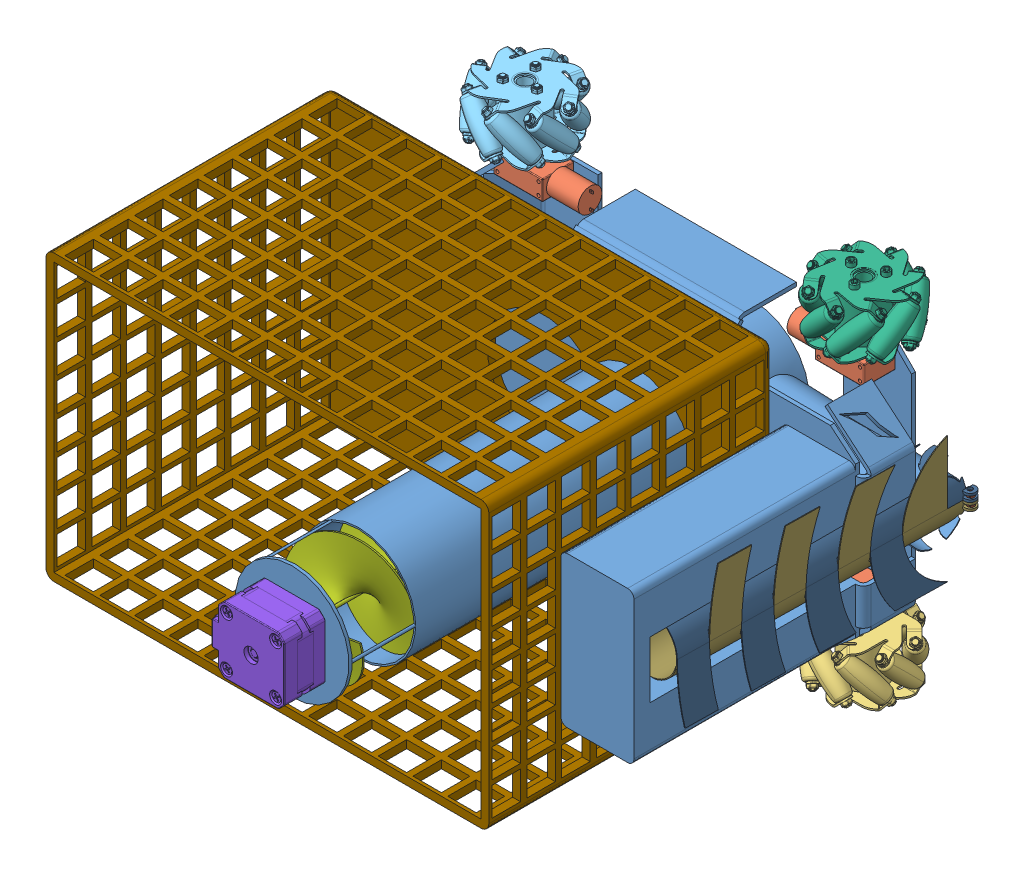
SolidWorks assembly tennis_car2, configuration 默认. Lengths in mm.
Overall size (342.44 226.19 334.2).
20 component instances, 12 part files, 28 mates.
Components (placement in the parent):
- car_main_body-1: car_main_body [默认] at (-145.051 -370.0736 71.4729) x (0 1 0) z (0 0 1) size (155.3 280.48 291.54)
- RF-1: RF [默认] at (73.9859 -396.0617 -100.86) size (72.83 55.75 59.47)
  - DC-1: DC [默认] at (11.5455 -40.5143 8.3808) x (-1 0 0) z (0 -1 0) size (53.09 20 29.75)
  - Mecanum_wheel_RF-1: Mecanum_wheel_RF [默认] at (50.073 -104.5143 -58.7387) x (0 1 0) z (0 0 1) size (37 59.47 59.47)
- RB-1: RB [默认] at (-99.6113 -409.5895 -127.3135) size (85.22 55.84 84.26)
  - DC-1: DC [默认] at (0.8482 -26.9825 34.8343) x (1 0 0) z (0 -1 0) size (53.09 20 29.75)
  - Mecanum_wheel_RB2-1: Mecanum_wheel_RB2 [默认] at (-29.583 -87.0073 9.2199) x (0 -1 0) z (0.536613 0 0.843828) size (37 61.04 61.04)
- LB-1: LB [默认] at (-105.6209 -285.1235 -91.7022) size (78.74 55.75 71.3)
  - DC-1: DC [默认] at (6.8577 -59.4516 -0.777) x (1 0 0) z (0 1 0) size (53.09 20 29.75)
  - Mecanum_wheel_LB2-1: Mecanum_wheel_LB2 [默认] at (-16.0195 4.5484 -71.463) x (0 -1 0) z (-0.224244 0 0.974533) size (37 59.47 59.47)
- LF-1: LF [默认] at (100.0091 -244.6315 -121.7936) size (85.57 55.84 84.97)
  - DC-1: DC [默认] at (-14.4777 -99.9396 29.3144) x (-1 0 0) z (0 1 0) size (53.09 20 29.75)
  - Mecanum_wheel_LF2-1: Mecanum_wheel_LF2 [默认] at (24.6483 -39.9149 11.6464) x (0 1 0) z (-0.82086 0 0.571129) size (37 61.04 61.04)
- spiral_tube-1: spiral_tube [默认] at (4.7184 -390.5736 -116.766) x (0.166187 -0.986094 0) z (0 0 1) size (68 68 282.11)
- Stepper Motor3-1: Stepper Motor3 [默认] at (4.7184 -390.5736 198.234) x (0 1 0) z (-1 0 0) size (42 43 47.1)
- box2-1: box2 [默认] at (-52.9088 -300.5736 41.234) x (1 0 0) z (0 -1 0) size (280 180 180)
- 夹爪-1: 夹爪 [默认] at (126.3983 -390.5736 -113.4559) x (0 1 0) z (-0.017044 0 0.999855) size (58.5 41.56 184.56)
- connection1-1: connection1 [默认] at (140.8179 -393.0736 -113.3823) x (0.999248 0 0.038769) z (0.038769 0 -0.999248) size (9.12 3 4.5)
- connection1-2: connection1 [默认] at (140.8179 -388.0736 -113.3823) x (0.999248 0 0.038769) z (0.038769 0 -0.999248) size (9.12 3 4.5)
- 夹爪2-1: 夹爪2 [默认] at (126.3983 -390.5736 -113.4559) x (0 1 0) z (-0.017044 0 0.999855) size (58.5 41.56 184.56)
Mates (geometry in assembly coordinates):
- 重合1: coincident anti-aligned: plane of RF-1/DC-1 through (110.5314 -436.576 -102.4792) normal (0 0 -1); plane of car_main_body-1 through (100.4806 -390.5736 -102.4792) normal (0 0 1)
- 重合2: coincident aligned: plane of car_main_body-1 through (-145.051 -461.576 71.4729) normal (0 -1 0); plane of RF-1/DC-1 through (85.5314 -461.576 -92.4792) normal (0 -1 0)
- 重合3: coincident: line of car_main_body-1 through (110.5314 -461.576 -104.9792) axis (0 0 1); plane of RF-1/DC-1 through (110.5314 -461.576 -107.4792) normal (1 0 0)
- 重合4: coincident anti-aligned: plane of car_main_body-1 through (-91.0439 -390.5736 -102.4792) normal (0 0 1); plane of RB-1/DC-1 through (-123.7631 -436.5721 -102.4792) normal (0 0 -1)
- 重合5: coincident aligned: plane of car_main_body-1 through (-123.6589 -461.5721 -103.9928) normal (0 -1 0); plane of RB-1/DC-1 through (-98.7631 -461.5721 -92.4792) normal (0 -1 0)
- 重合6: coincident: line of car_main_body-1 through (-123.7631 -445.1021 -102.4792) axis (0 -1 0); plane of RB-1/DC-1 through (-123.7631 -461.5721 -77.4792) normal (-1 0 0)
- 重合7: coincident anti-aligned: plane of car_main_body-1 through (-91.0439 -390.5736 -102.4792) normal (0 0 1); plane of LB-1/DC-1 through (-123.7631 -344.5751 -102.4792) normal (0 0 -1)
- 重合8: coincident aligned: plane of car_main_body-1 through (-125.6782 -319.5751 -101.5862) normal (0 1 0); plane of LB-1/DC-1 through (-98.7631 -319.5751 -92.4792) normal (0 1 0)
- 重合9: coincident: line of car_main_body-1 through (-123.7631 -319.5751 -102.4792) axis (0 -1 0); plane of LB-1/DC-1 through (-123.7631 -319.5751 -107.4792) normal (-1 0 0)
- 重合10: coincident anti-aligned: plane of car_main_body-1 through (100.4806 -390.5736 -102.4792) normal (0 0 1); plane of LF-1/DC-1 through (110.5314 -344.5712 -102.4792) normal (0 0 -1)
- 重合11: coincident aligned: plane of car_main_body-1 through (-145.051 -319.5712 71.4729) normal (0 1 0); plane of LF-1/DC-1 through (85.5314 -319.5712 -92.4792) normal (0 1 0)
- 重合12: coincident: line of car_main_body-1 through (110.5314 -319.5712 -102.4792) axis (0 0 -1); plane of LF-1/DC-1 through (110.5314 -319.5712 -77.4792) normal (1 0 0)
- 同心1: concentric aligned: cylinder of car_main_body-1 through (4.7184 -390.5736 171.234) axis (0 0 -1) radius 36; cylinder of spiral_tube-1 through (4.7184 -390.5736 165.234) axis (0 0 -1) radius 1
- 重合13: coincident anti-aligned: plane of car_main_body-1 through (4.7184 -390.5736 -116.766) normal (0 0 1); plane of spiral_tube-1 through (4.7184 -390.5736 -116.766) normal (0 0 -1)
- 同心2: concentric aligned: cylinder of car_main_body-1 through (4.7184 -390.5736 171.234) axis (0 0 1) radius 11; cylinder of Stepper Motor3-1 through (4.7184 -390.5736 155.234) axis (0 0 1) radius 2.5
- 同心3: concentric aligned: circle of car_main_body-1; cone of Stepper Motor3-1 through (20.2184 -375.0736 173.234) axis (0 0 1)
- 重合16: coincident anti-aligned: plane of car_main_body-1 through (4.7184 -390.5736 173.234) normal (0 0 1); plane of Stepper Motor3-1 through (4.7184 -390.5736 173.234) normal (0 0 -1)
- 重合17: coincident anti-aligned: plane of car_main_body-1 through (4.7184 -390.5736 -48.766) normal (0 0 1); plane of box2-1 through (-192.9088 -480.5736 -48.766) normal (0 0 -1)
- 重合18: coincident aligned: plane of car_main_body-1 through (-145.051 -390.5736 71.4729) normal (0 -1 0); plane of box2-1 through (-52.9088 -390.5736 41.234) normal (0 -1 0)
- 同心4: concentric anti-aligned: cylinder of car_main_body-1 through (129.4557 -393.0736 179.4723) axis (0.038769 0 -0.999248) radius 1; cylinder of connection1-1 through (140.8955 -393.0736 -115.3808) axis (-0.038769 0 0.999248) radius 1
- 重合20: coincident aligned: plane of car_main_body-1 through (140.8955 -393.0736 -115.3808) normal (0.038769 0 -0.999248); plane of connection1-1 through (140.8955 -393.0736 -115.3808) normal (0.038769 0 -0.999248)
- 同心5: concentric anti-aligned: cylinder of car_main_body-1 through (129.4557 -388.0736 179.4723) axis (0.038769 0 -0.999248) radius 1; cylinder of connection1-2 through (140.8955 -388.0736 -115.3808) axis (-0.038769 0 0.999248) radius 1
- 重合22: coincident aligned: plane of car_main_body-1 through (140.8955 -388.0736 -115.3808) normal (0.038769 0 -0.999248); plane of connection1-2 through (140.8955 -388.0736 -115.3808) normal (0.038769 0 -0.999248)
- 重合23: coincident aligned: circle of 夹爪-1; cylinder of connection1-2 through (145.9742 -389.0736 -114.183) axis (0 1 0) radius 1.5
- 重合24: coincident anti-aligned: plane of 夹爪-1 through (145.9742 -389.0736 -114.183) normal (0 1 0); plane of connection1-2 through (145.9742 -389.0736 -114.183) normal (0 -1 0)
- 同心6: concentric aligned: cylinder of 夹爪2-1 through (145.9742 -385.5736 -114.183) axis (0 -1 0) radius 1.5; circle of connection1-1
- 重合26: coincident anti-aligned: plane of connection1-1; plane of 夹爪2-1
- 重合27: coincident aligned: plane of 夹爪-1 through (142.1686 -430.5736 46.8362) normal (0.999855 0 0.017044); plane of 夹爪2-1 through (142.5094 -350.5736 26.8391) normal (0.999855 0 0.017044)
